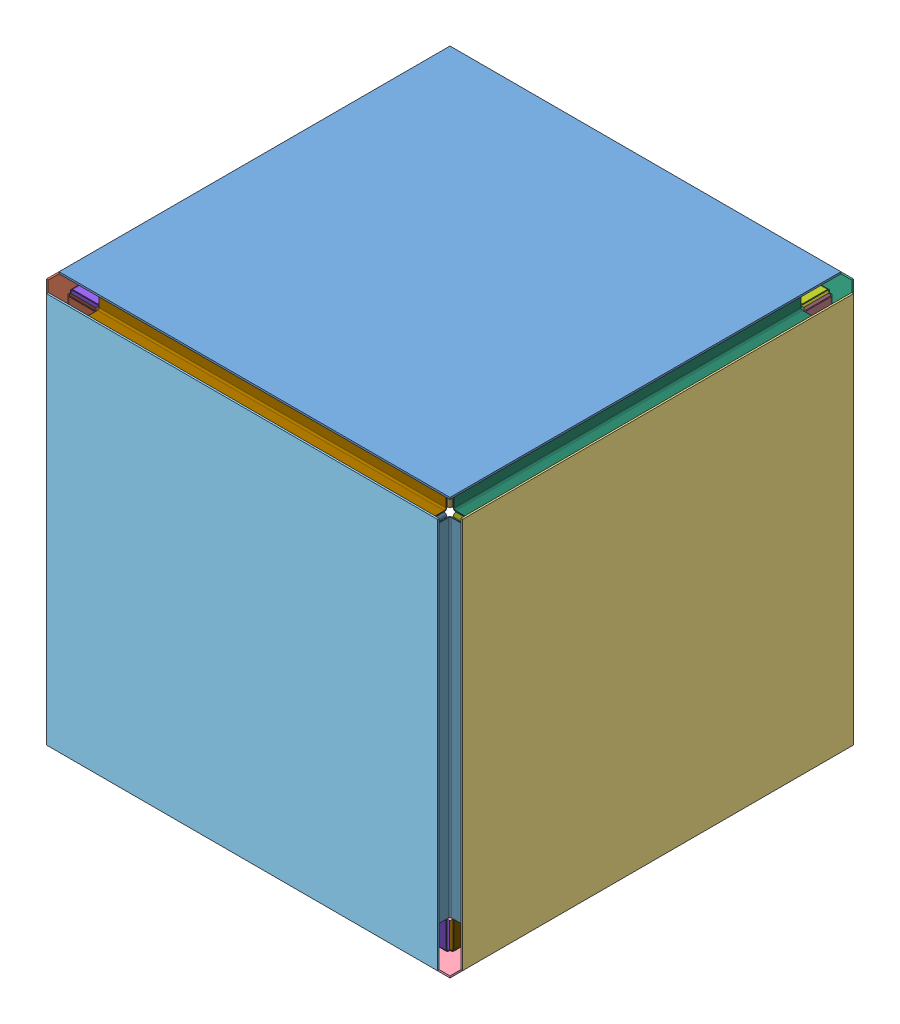
SolidWorks assembly cube_33, configuration cube33. Lengths in mm.
Overall size (366.4 366.4 366.4).
30 component instances, 30 part files, 93 mates.
Components (placement in the parent):
- pr^cube_33-28: pr^cube_33 [cube01] x (-1 0 0) z (0 0 1) size (344.17 1.59 344.17) (virtual)
- pg^cube_33-20: pg^cube_33 [cube01] x (0 -1 0) z (0 0 1) size (344.17 1.59 344.17) (virtual)
- po^cube_33-22: po^cube_33 [cube01] x (0 1 0) z (0 0 1) size (344.17 1.59 344.17) (virtual)
- py^cube_33-21: py^cube_33 [cube01] at origin size (344.17 1.59 344.17) (virtual)
- pc^cube_33-18: pc^cube_33 [cube01] x (-1 0 0) z (0 -1 0) size (344.17 1.59 344.17) (virtual)
- pb^cube_33-21: pb^cube_33 [cube01] x (-1 0 0) z (0 1 0) size (344.17 1.59 344.17) (virtual)
- br1^cube_33-49: br1^cube_33 [Default] at (0 156.21 -156.21) x (0 0 1) z (-1 0 0) size (50.8 50.8 305.31) (virtual)
- br2^cube_33-61: br2^cube_33 [Default] at (-156.21 156.21 0) size (50.8 50.8 305.31) (virtual)
- br3^cube_33-46: br3^cube_33 [Default] at (0 156.21 156.21) x (0 0 -1) z (1 0 0) size (50.8 50.8 305.31) (virtual)
- bg1^cube_33-47: bg1^cube_33 [Default] at (-156.21 -156.21 0) x (0 1 0) z (0 0 1) size (50.8 50.8 305.31) (virtual)
- bg2^cube_33-44: bg2^cube_33 [Default] at (-156.21 0 156.21) x (0 0 -1) z (0 1 0) size (50.8 50.8 305.31) (virtual)
- bg3^cube_33-40: bg3^cube_33 [Default] at (-156.21 0 -156.21) x (0 0 1) z (0 -1 0) size (50.8 50.8 305.31) (virtual)
- bo1^cube_33-42: bo1^cube_33 [Default] at (156.21 0 -156.21) x (0 0 1) z (0 1 0) size (50.8 50.8 305.31) (virtual)
- bo2^cube_33-46: bo2^cube_33 [Default] at (156.21 0 156.21) x (0 0 -1) z (0 -1 0) size (50.8 50.8 305.31) (virtual)
- bo3^cube_33-62: bo3^cube_33 [Default] at (156.21 156.21 0) x (0 -1 0) z (0 0 1) size (50.8 50.8 305.31) (virtual)
- by1^cube_33-41: by1^cube_33 [Default] at (0 -156.21 -156.21) x (0 0 1) z (1 0 0) size (50.8 50.8 305.31) (virtual)
- by2^cube_33-45: by2^cube_33 [Default] at (0 -156.21 156.21) x (0 0 -1) z (-1 0 0) size (50.8 50.8 305.31) (virtual)
- by3^cube_33-48: by3^cube_33 [Default] at (156.21 -156.21 0) x (-1 0 0) z (0 0 1) size (50.8 50.8 305.31) (virtual)
- dr1^cube_33-55: dr1^cube_33 [cube01] at (-181.0046 181.61 0) x (0 -1 0) z (0 0 1) size (26.01 26.01 363.23) (hidden, virtual)
- dr2^cube_33-37: dr2^cube_33 [cube01] at (0 181.61 181.0046) x (0 -1 0) z (1 0 0) size (26.01 26.01 363.23) (hidden, virtual)
- dr3^cube_33-33: dr3^cube_33 [cube01] at (0 181.61 -181.0046) x (0 -1 0) z (-1 0 0) size (26.01 26.01 363.23) (hidden, virtual)
- dg1^cube_33-38: dg1^cube_33 [cube01] at (-181.61 0 181.0046) x (1 0 0) z (0 1 0) size (26.01 26.01 363.23) (hidden, virtual)
- dg2^cube_33-41: dg2^cube_33 [cube01] at (-181.61 -181.0046 0) size (26.01 26.01 363.23) (hidden, virtual)
- dg3^cube_33-34: dg3^cube_33 [cube01] at (-181.61 0 -181.0046) x (1 0 0) z (0 -1 0) size (26.01 26.01 363.23) (hidden, virtual)
- do3^cube_33-47: do3^cube_33 [cube01] at (181.61 181.0046 0) x (-1 0 0) z (0 0 1) size (26.01 26.01 363.23) (hidden, virtual)
- do1^cube_33-36: do1^cube_33 [cube01] at (181.61 0 -181.0046) x (-1 0 0) z (0 1 0) size (26.01 26.01 363.23) (hidden, virtual)
- do2^cube_33-40: do2^cube_33 [cube01] at (181.61 0 181.0046) x (-1 0 0) z (0 -1 0) size (26.01 26.01 363.23) (hidden, virtual)
- dy1^cube_33-35: dy1^cube_33 [cube01] at (0 -181.61 -181.0046) x (0 1 0) z (1 0 0) size (26.01 26.01 363.23) (hidden, virtual)
- dy2^cube_33-39: dy2^cube_33 [cube01] at (0 -181.61 181.0046) x (0 1 0) z (-1 0 0) size (26.01 26.01 363.23) (hidden, virtual)
- dy3^cube_33-42: dy3^cube_33 [cube01] at (181.0046 -181.61 0) x (0 1 0) z (0 0 1) size (26.01 26.01 363.23) (hidden, virtual)
Mates (geometry in assembly coordinates):
- Coincident1: coincident anti-aligned: plane of pr^cube_33-28 through (172.085 181.61 -172.085) normal (0 -1 0); plane of br1^cube_33-49 through (-152.654 181.61 -156.21) normal (0 1 0)
- Coincident2: coincident anti-aligned: plane of pr^cube_33-28 through (172.085 181.61 -172.085) normal (0 -1 0); plane of br2^cube_33-61 through (-156.21 181.61 152.654) normal (0 1 0)
- Coincident3: coincident anti-aligned: plane of pr^cube_33-28 through (172.085 181.61 -172.085) normal (0 -1 0); plane of br3^cube_33-46 through (152.654 181.61 156.21) normal (0 1 0)
- Coincident4: coincident anti-aligned: plane of pr^cube_33-28 through (172.085 181.61 -172.085) normal (0 -1 0); plane of bo3^cube_33-62 through (156.21 181.61 152.654) normal (0 1 0)
- Coincident5: coincident anti-aligned: plane of pr^cube_33-28 through (172.085 181.61 -172.085) normal (0 -1 0); plane of dr3^cube_33-33 through (0 181.61 -362.6146) normal (0 1 0)
- Coincident6: coincident anti-aligned: plane of pr^cube_33-28 through (172.085 181.61 -172.085) normal (0 -1 0); plane of dr1^cube_33-55 through (-362.6146 181.61 0) normal (0 1 0)
- Coincident7: coincident anti-aligned: plane of pr^cube_33-28 through (172.085 181.61 -172.085) normal (0 -1 0); plane of do3^cube_33-47 through (-0.6054 181.61 0) normal (0 1 0)
- Coincident8: coincident anti-aligned: plane of pr^cube_33-28 through (172.085 181.61 -172.085) normal (0 -1 0); plane of dr2^cube_33-37 through (0 181.61 362.6146) normal (0 1 0)
- Coincident34: coincident anti-aligned: plane of pb^cube_33-21 through (172.085 -172.085 -181.61) normal (0 0 1); plane of by1^cube_33-41 through (152.654 -156.21 -181.61) normal (0 0 -1)
- Coincident35: coincident anti-aligned: plane of pb^cube_33-21 through (172.085 -172.085 -181.61) normal (0 0 1); plane of bo1^cube_33-42 through (156.21 152.654 -181.61) normal (0 0 -1)
- Coincident36: coincident anti-aligned: plane of pb^cube_33-21 through (172.085 -172.085 -181.61) normal (0 0 1); plane of br1^cube_33-49 through (-152.654 156.21 -181.61) normal (0 0 -1)
- Coincident37: coincident anti-aligned: plane of pb^cube_33-21 through (172.085 -172.085 -181.61) normal (0 0 1); plane of bg3^cube_33-40 through (-156.21 -152.654 -181.61) normal (0 0 -1)
- Coincident38: coincident anti-aligned: plane of pb^cube_33-21 through (172.085 -172.085 -181.61) normal (0 0 1); plane of dg3^cube_33-34 through (0.6054 0 -181.61) normal (0 0 -1)
- Coincident39: coincident anti-aligned: plane of pb^cube_33-21 through (172.085 -172.085 -181.61) normal (0 0 1); plane of dr3^cube_33-33 through (0 -0.6054 -181.61) normal (0 0 -1)
- Coincident40: coincident anti-aligned: plane of pb^cube_33-21 through (172.085 -172.085 -181.61) normal (0 0 1); plane of do1^cube_33-36 through (-0.6054 0 -181.61) normal (0 0 -1)
- Coincident41: coincident anti-aligned: plane of pb^cube_33-21 through (172.085 -172.085 -181.61) normal (0 0 1); plane of dy1^cube_33-35 through (0 0.6054 -181.61) normal (0 0 -1)
- Coincident42: coincident anti-aligned: plane of pc^cube_33-18 through (172.085 172.085 181.61) normal (0 0 -1); plane of bo2^cube_33-46 through (156.21 -152.654 181.61) normal (0 0 1)
- Coincident43: coincident anti-aligned: plane of pc^cube_33-18 through (172.085 172.085 181.61) normal (0 0 -1); plane of br3^cube_33-46 through (152.654 156.21 181.61) normal (0 0 1)
- Coincident44: coincident anti-aligned: plane of pc^cube_33-18 through (172.085 172.085 181.61) normal (0 0 -1); plane of bg2^cube_33-44 through (-156.21 152.654 181.61) normal (0 0 1)
- Coincident45: coincident anti-aligned: plane of pc^cube_33-18 through (172.085 172.085 181.61) normal (0 0 -1); plane of by2^cube_33-45 through (-152.654 -156.21 181.61) normal (0 0 1)
- Coincident46: coincident anti-aligned: plane of pc^cube_33-18 through (172.085 172.085 181.61) normal (0 0 -1); plane of do2^cube_33-40 through (-0.6054 0 181.61) normal (0 0 1)
- Coincident47: coincident anti-aligned: plane of pc^cube_33-18 through (172.085 172.085 181.61) normal (0 0 -1); plane of dy2^cube_33-39 through (0 0.6054 181.61) normal (0 0 1)
- Coincident48: coincident anti-aligned: plane of pc^cube_33-18 through (172.085 172.085 181.61) normal (0 0 -1); plane of dg1^cube_33-38 through (0.6054 0 181.61) normal (0 0 1)
- Coincident49: coincident anti-aligned: plane of pc^cube_33-18 through (172.085 172.085 181.61) normal (0 0 -1); plane of dr2^cube_33-37 through (0 -0.6054 181.61) normal (0 0 1)
- Coincident50: coincident anti-aligned: plane of pg^cube_33-20 through (-181.61 172.085 -172.085) normal (1 0 0); plane of bg3^cube_33-40 through (-181.61 -152.654 -156.21) normal (-1 0 0)
- Coincident51: coincident anti-aligned: plane of pg^cube_33-20 through (-181.61 172.085 -172.085) normal (1 0 0); plane of bg1^cube_33-47 through (-181.61 -156.21 152.654) normal (-1 0 0)
- Coincident52: coincident anti-aligned: plane of pg^cube_33-20 through (-181.61 172.085 -172.085) normal (1 0 0); plane of bg2^cube_33-44 through (-181.61 152.654 156.21) normal (-1 0 0)
- Coincident53: coincident anti-aligned: plane of pg^cube_33-20 through (-181.61 172.085 -172.085) normal (1 0 0); plane of dr1^cube_33-55 through (-181.61 -0.6054 0) normal (-1 0 0)
- Coincident54: coincident anti-aligned: plane of pg^cube_33-20 through (-181.61 172.085 -172.085) normal (1 0 0); plane of dg3^cube_33-34 through (-181.61 0 -362.6146) normal (-1 0 0)
- Coincident55: coincident anti-aligned: plane of pg^cube_33-20 through (-181.61 172.085 -172.085) normal (1 0 0); plane of dg2^cube_33-41 through (-181.61 -362.6146 0) normal (-1 0 0)
- Coincident56: coincident anti-aligned: plane of pg^cube_33-20 through (-181.61 172.085 -172.085) normal (1 0 0); plane of dg1^cube_33-38 through (-181.61 0 362.6146) normal (-1 0 0)
- Coincident99: coincident anti-aligned: plane of pg^cube_33-20 through (-181.61 172.085 -172.085) normal (1 0 0); plane of br2^cube_33-61 through (-181.61 156.21 152.654) normal (-1 0 0)
- Coincident57: coincident anti-aligned: plane of py^cube_33-21 through (-172.085 -181.61 -172.085) normal (0 1 0); plane of by3^cube_33-48 through (156.21 -181.61 152.654) normal (0 -1 0)
- Coincident58: coincident anti-aligned: plane of py^cube_33-21 through (-172.085 -181.61 -172.085) normal (0 1 0); plane of by2^cube_33-45 through (-152.654 -181.61 156.21) normal (0 -1 0)
- Coincident59: coincident anti-aligned: plane of py^cube_33-21 through (-172.085 -181.61 -172.085) normal (0 1 0); plane of bg1^cube_33-47 through (-156.21 -181.61 152.654) normal (0 -1 0)
- Coincident60: coincident anti-aligned: plane of py^cube_33-21 through (-172.085 -181.61 -172.085) normal (0 1 0); plane of by1^cube_33-41 through (152.654 -181.61 -156.21) normal (0 -1 0)
- Coincident61: coincident anti-aligned: plane of py^cube_33-21 through (-172.085 -181.61 -172.085) normal (0 1 0); plane of dy3^cube_33-42 through (362.6146 -181.61 0) normal (0 -1 0)
- Coincident62: coincident anti-aligned: plane of py^cube_33-21 through (-172.085 -181.61 -172.085) normal (0 1 0); plane of dy2^cube_33-39 through (0 -181.61 362.6146) normal (0 -1 0)
- Coincident63: coincident anti-aligned: plane of py^cube_33-21 through (-172.085 -181.61 -172.085) normal (0 1 0); plane of dg2^cube_33-41 through (0.6054 -181.61 0) normal (0 -1 0)
- Coincident64: coincident anti-aligned: plane of py^cube_33-21 through (-172.085 -181.61 -172.085) normal (0 1 0); plane of dy1^cube_33-35 through (0 -181.61 -362.6146) normal (0 -1 0)
- Coincident65: coincident anti-aligned: plane of po^cube_33-22 through (181.61 -172.085 -172.085) normal (-1 0 0); plane of bo1^cube_33-42 through (181.61 152.654 -156.21) normal (1 0 0)
- Coincident66: coincident anti-aligned: plane of po^cube_33-22 through (181.61 -172.085 -172.085) normal (-1 0 0); plane of by3^cube_33-48 through (181.61 -156.21 152.654) normal (1 0 0)
- Coincident67: coincident anti-aligned: plane of po^cube_33-22 through (181.61 -172.085 -172.085) normal (-1 0 0); plane of bo2^cube_33-46 through (181.61 -152.654 156.21) normal (1 0 0)
- Coincident68: coincident anti-aligned: plane of po^cube_33-22 through (181.61 -172.085 -172.085) normal (-1 0 0); plane of bo3^cube_33-62 through (181.61 156.21 152.654) normal (1 0 0)
- Coincident69: coincident anti-aligned: plane of po^cube_33-22 through (181.61 -172.085 -172.085) normal (-1 0 0); plane of do2^cube_33-40 through (181.61 0 362.6146) normal (1 0 0)
- Coincident70: coincident anti-aligned: plane of po^cube_33-22 through (181.61 -172.085 -172.085) normal (-1 0 0); plane of do3^cube_33-47 through (181.61 362.6146 0) normal (1 0 0)
- Coincident71: coincident anti-aligned: plane of po^cube_33-22 through (181.61 -172.085 -172.085) normal (-1 0 0); plane of do1^cube_33-36 through (181.61 0 -362.6146) normal (1 0 0)
- Coincident72: coincident anti-aligned: plane of po^cube_33-22 through (181.61 -172.085 -172.085) normal (-1 0 0); plane of dy3^cube_33-42 through (181.61 0.6054 0) normal (1 0 0)
- Coincident73: coincident aligned: plane of assembly through (0 0 0) normal (0 0 1); plane of dy3^cube_33-42 through (181.0046 -181.61 0) normal (0 0 1)
- Coincident74: coincident aligned: plane of assembly through (0 0 0) normal (0 0 1); plane of by3^cube_33-48 through (156.21 -156.21 0) normal (0 0 1)
- Coincident75: coincident aligned: plane of assembly through (0 0 0) normal (0 0 1); plane of bo3^cube_33-62 through (156.21 156.21 0) normal (0 0 1)
- Coincident76: coincident aligned: plane of assembly through (0 0 0) normal (0 0 1); plane of do3^cube_33-47 through (181.61 181.0046 0) normal (0 0 1)
- Coincident77: coincident aligned: plane of assembly through (0 0 0) normal (0 0 1); plane of dg2^cube_33-41 through (-181.61 -181.0046 0) normal (0 0 1)
- Coincident78: coincident aligned: plane of assembly through (0 0 0) normal (0 0 1); plane of bg1^cube_33-47 through (-156.21 -156.21 0) normal (0 0 1)
- Coincident79: coincident aligned: plane of assembly through (0 0 0) normal (0 0 1); plane of dr1^cube_33-55 through (-181.0046 181.61 0) normal (0 0 1)
- Coincident80: coincident aligned: plane of assembly through (0 0 0) normal (0 0 1); plane of br2^cube_33-61 through (-156.21 156.21 0) normal (0 0 1)
- Coincident81: coincident aligned: plane of assembly through (0 0 0) normal (0 1 0); plane of bo1^cube_33-42 through (156.21 0 -156.21) normal (0 1 0)
- Coincident82: coincident aligned: plane of assembly through (0 0 0) normal (0 1 0); plane of py^cube_33-21 through (0 0 0) normal (0 1 0)
- Coincident83: coincident aligned: plane of assembly through (0 0 0) normal (0 1 0); plane of do1^cube_33-36 through (181.61 0 -181.0046) normal (0 1 0)
- Coincident84: coincident anti-aligned: plane of assembly through (0 0 0) normal (0 1 0); plane of bg3^cube_33-40 through (-156.21 0 -156.21) normal (0 -1 0)
- Coincident85: coincident anti-aligned: plane of assembly through (0 0 0) normal (0 1 0); plane of dg3^cube_33-34 through (-181.61 0 -181.0046) normal (0 -1 0)
- Coincident86: coincident aligned: plane of assembly through (0 0 0) normal (0 1 0); plane of dg1^cube_33-38 through (-181.61 0 181.0046) normal (0 1 0)
- Coincident87: coincident aligned: plane of assembly through (0 0 0) normal (0 1 0); plane of bg2^cube_33-44 through (-156.21 0 156.21) normal (0 1 0)
- Coincident88: coincident anti-aligned: plane of assembly through (0 0 0) normal (0 1 0); plane of bo2^cube_33-46 through (156.21 0 156.21) normal (0 -1 0)
- Coincident89: coincident anti-aligned: plane of assembly through (0 0 0) normal (0 1 0); plane of do2^cube_33-40 through (181.61 0 181.0046) normal (0 -1 0)
- Coincident90: coincident anti-aligned: plane of assembly through (0 0 0) normal (1 0 0); plane of by2^cube_33-45 through (0 -156.21 156.21) normal (-1 0 0)
- Coincident91: coincident anti-aligned: plane of assembly through (0 0 0) normal (1 0 0); plane of dy2^cube_33-39 through (0 -181.61 181.0046) normal (-1 0 0)
- Coincident92: coincident aligned: plane of assembly through (0 0 0) normal (1 0 0); plane of pg^cube_33-20
- Coincident93: coincident aligned: plane of assembly through (0 0 0) normal (1 0 0); plane of dr2^cube_33-37 through (0 181.61 181.0046) normal (1 0 0)
- Coincident94: coincident aligned: plane of assembly through (0 0 0) normal (1 0 0); plane of br3^cube_33-46 through (0 156.21 156.21) normal (1 0 0)
- Coincident95: coincident anti-aligned: plane of assembly through (0 0 0) normal (1 0 0); plane of dr3^cube_33-33 through (0 181.61 -181.0046) normal (-1 0 0)
- Coincident96: coincident anti-aligned: plane of assembly through (0 0 0) normal (1 0 0); plane of br1^cube_33-49 through (0 156.21 -156.21) normal (-1 0 0)
- Coincident97: coincident aligned: plane of assembly through (0 0 0) normal (1 0 0); plane of by1^cube_33-41 through (0 -156.21 -156.21) normal (1 0 0)
- Coincident98: coincident aligned: plane of assembly through (0 0 0) normal (1 0 0); plane of dy1^cube_33-35 through (0 -181.61 -181.0046) normal (1 0 0)
- Coincident100: coincident anti-aligned: plane of pr^cube_33-28; plane of assembly through (0 0 0) normal (1 0 0)
- Coincident101: coincident aligned: plane of pr^cube_33-28 through (0 0 0) normal (0 0 1); plane of assembly through (0 0 0) normal (0 0 1)
- Coincident102: coincident anti-aligned: plane of pr^cube_33-28; plane of assembly through (0 0 0) normal (0 1 0)
- Coincident106: coincident anti-aligned: plane of pg^cube_33-20; plane of assembly through (0 0 0) normal (0 1 0)
- Coincident107: coincident aligned: plane of pg^cube_33-20; plane of assembly through (0 0 0) normal (1 0 0)
- Coincident108: coincident aligned: plane of pg^cube_33-20 through (0 0 0) normal (0 0 1); plane of assembly through (0 0 0) normal (0 0 1)
- Coincident109: coincident aligned: plane of py^cube_33-21 through (0 0 0) normal (0 0 1); plane of assembly through (0 0 0) normal (0 0 1)
- Coincident110: coincident aligned: plane of py^cube_33-21 through (0 0 0) normal (0 1 0); plane of assembly through (0 0 0) normal (0 1 0)
- Coincident111: coincident aligned: plane of py^cube_33-21 through (0 0 0) normal (1 0 0); plane of assembly through (0 0 0) normal (1 0 0)
- Coincident112: coincident aligned: plane of po^cube_33-22 through (0 0 0) normal (0 0 1); plane of assembly through (0 0 0) normal (0 0 1)
- Coincident113: coincident anti-aligned: plane of po^cube_33-22; plane of assembly through (0 0 0) normal (1 0 0)
- Coincident114: coincident aligned: plane of po^cube_33-22; plane of assembly through (0 0 0) normal (0 1 0)
- Coincident115: coincident anti-aligned: plane of pc^cube_33-18 through (0 0 0) normal (0 -1 0); plane of assembly through (0 0 0) normal (0 1 0)
- Coincident116: coincident anti-aligned: plane of pc^cube_33-18; plane of assembly through (0 0 0) normal (0 0 1)
- Coincident117: coincident anti-aligned: plane of pc^cube_33-18; plane of assembly through (0 0 0) normal (1 0 0)
- Coincident118: coincident aligned: plane of pb^cube_33-21 through (0 0 0) normal (0 1 0); plane of assembly through (0 0 0) normal (0 1 0)
- Coincident119: coincident aligned: plane of pb^cube_33-21; plane of assembly through (0 0 0) normal (0 0 1)
- Coincident120: coincident anti-aligned: line of pb^cube_33-21 through (0.8731 -0.8731 0) axis (0 0 -1); sketch_entity of pr^cube_33-28; plane of pb^cube_33-21 through (172.085 -172.085 -183.1975) normal (0 0 -1); plane of py^cube_33-21 through (-172.085 -183.1975 -172.085) normal (0 -1 0)
- cyan_cut: unknown: unknown of pc^cube_33-18; plane of pc^cube_33-18 through (172.085 172.085 183.1975) normal (0 0 1); plane of pg^cube_33-20 through (-183.1975 172.085 -172.085) normal (-1 0 0); plane of po^cube_33-22 through (183.1975 -172.085 -172.085) normal (1 0 0)
